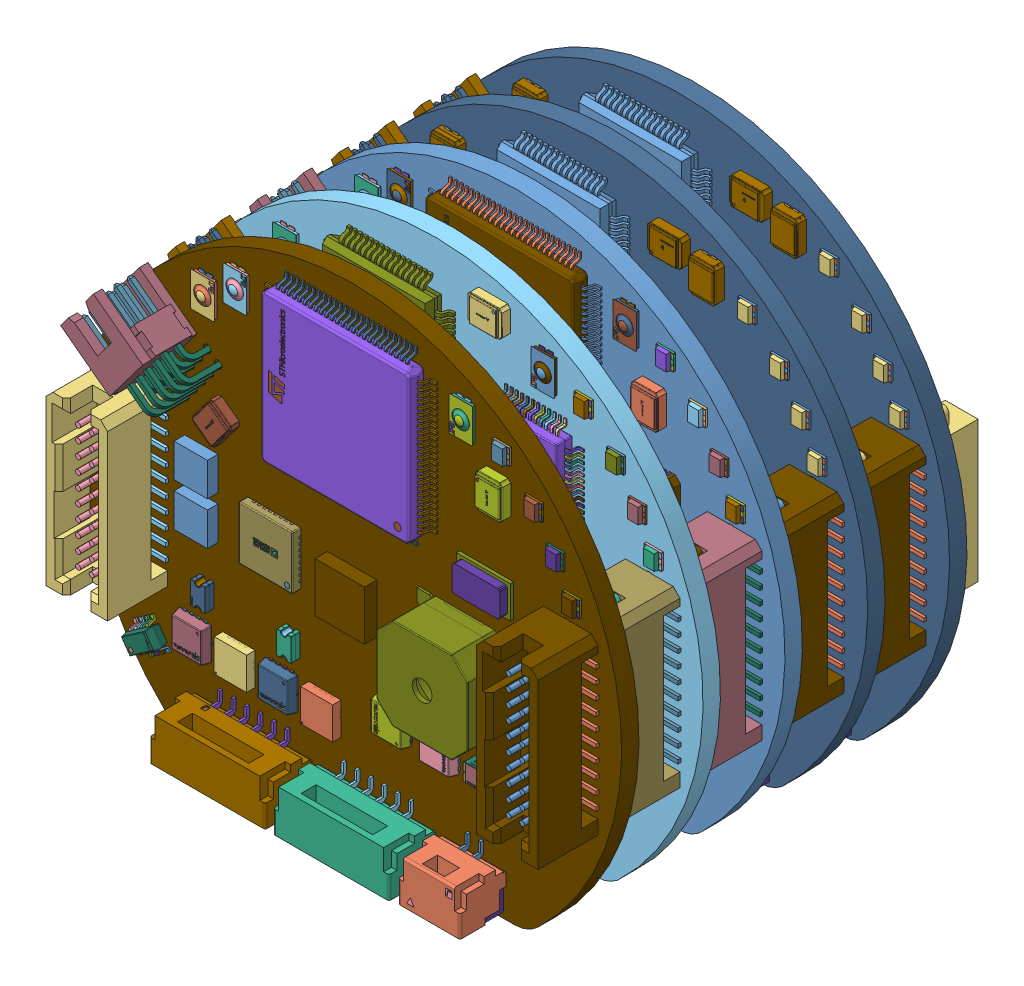
SolidWorks assembly ASSY_HYDRA_MASTER, configuration Default. Lengths in mm. (continued)
Components (placement in the parent): (continued)
- HYDRA_V4_RECOVERY-1: HYDRA_V4_RECOVERY [Default] at (-0.0049 -0.0019 15.2232) size (50.1 44.1 11.77) (continued)
  - Open CASCADE STEP translator 7.5 3383-1: Open CASCADE STEP translator 7.5 3383 [Default] at origin size (2 3 0.57)
  - Open CASCADE STEP translator 7.5 3384-1: Open CASCADE STEP translator 7.5 3384 [Default] at origin size (2.2 3.2 0.32)
  - Open CASCADE STEP translator 7.5 3385-1: Open CASCADE STEP translator 7.5 3385 [Default] at origin size (0.46 0.93 0.01)
  - Open CASCADE STEP translator 7.5 3386-1: Open CASCADE STEP translator 7.5 3386 [Default] at origin size (1.6 1.5 0.2)
  - Open CASCADE STEP translator 7.5 3387-1: Open CASCADE STEP translator 7.5 3387 [Default] at origin size (1.6 1.4 0.19)
  - Open CASCADE STEP translator 7.5 3388-1: Open CASCADE STEP translator 7.5 3388 [Default] at origin size (1.1 1.5 0.36)
  - Open CASCADE STEP translator 7.5 3389-1: Open CASCADE STEP translator 7.5 3389 [Default] at origin size (1.6 1.5 0.2)
  - Open CASCADE STEP translator 7.5 3390-1: Open CASCADE STEP translator 7.5 3390 [Default] at origin size (1.6 1.4 0.19)
  - Open CASCADE STEP translator 7.5 3391-1: Open CASCADE STEP translator 7.5 3391 [Default] at origin size (1.1 1.5 0.36)
  - Open CASCADE STEP translator 7.5 3392-1: Open CASCADE STEP translator 7.5 3392 [Default] at origin size (1.6 1.5 0.2)
  - Open CASCADE STEP translator 7.5 3393-1: Open CASCADE STEP translator 7.5 3393 [Default] at origin size (1.6 1.4 0.19)
  - Open CASCADE STEP translator 7.5 3394-1: Open CASCADE STEP translator 7.5 3394 [Default] at origin size (1.1 1.5 0.36)
  - Open CASCADE STEP translator 7.5 3395-1: Open CASCADE STEP translator 7.5 3395 [Default] at origin size (5.72 15.88 6.73)
  - Open CASCADE STEP translator 7.5 3396-1: Open CASCADE STEP translator 7.5 3396 [Default] at origin size (1.78 12.7 4.01)
  - Open CASCADE STEP translator 7.5 3397-1: Open CASCADE STEP translator 7.5 3397 [Default] at origin size (5.84 12.7 0.83)
  - Open CASCADE STEP translator 7.5 3398-1: Open CASCADE STEP translator 7.5 3398 [Default] at origin size (5.72 15.88 6.73)
  - Open CASCADE STEP translator 7.5 3399-1: Open CASCADE STEP translator 7.5 3399 [Default] at origin size (1.78 12.7 4.01)
  - Open CASCADE STEP translator 7.5 3400-1: Open CASCADE STEP translator 7.5 3400 [Default] at origin size (5.84 12.7 0.83)
  - Open CASCADE STEP translator 7.5 3401-1: Open CASCADE STEP translator 7.5 3401 [Default] at origin size (3.68 15.88 5.84)
  - Open CASCADE STEP translator 7.5 3402-1: Open CASCADE STEP translator 7.5 3402 [Default] at origin size (4.09 12.7 1.18)
  - Open CASCADE STEP translator 7.5 3403-1: Open CASCADE STEP translator 7.5 3403 [Default] at origin size (3.68 15.88 5.84)
  - Open CASCADE STEP translator 7.5 3404-1: Open CASCADE STEP translator 7.5 3404 [Default] at origin size (4.09 12.7 1.18)
- HYDRA_V4_POWER-1: HYDRA_V4_POWER [Default] at (-0.0043 -0.002 -7.6116) size (50.15 44.15 11.77)
  - Board-1: Board [Default] at origin size (50.15 44.15 1.61)
    - Open CASCADE STEP translator 7.5 2754.1.1-1: Open CASCADE STEP translator 7.5 2754.1.1 [Default] at (0 0 -1.6116) size (50.15 44.15 1.61)
  - J8-1: J8 [Default] at origin size (8.25 4.85 4.36)
    - Conn_JST_SM04B-GHS-TB_LF_SN_eec-1: Conn_JST_SM04B-GHS-TB_LF_SN_eec [Default] at (6.125 -14.4749 0.1) x (1 0 0) z (0 -1 0) size (8.25 4.36 4.85)
      - body-1: body [Default] at origin size (8.25 4.25 4.05)
      - Pins-1: Pins [Default] at origin size (7.65 2.05 4.85)
      - New Marking-1: New Marking [Default] at (-5.7821 4.251 3.7193) x (1 0 0) z (0 -1 0) size (0.46 0.67 0)
      - JST Logo-1: JST Logo [Default] at (14.4297 4.25 10.8095) x (1 0 0) z (0 1 0) size (1.76 0.68 0.01)
  - J7-1: J7 [Default] at origin size (9.7 4.86 4.36)
    - Conn_JST_SM05B-GHS-TB_LF_SN_eec-1: Conn_JST_SM05B-GHS-TB_LF_SN_eec [Default] at (11.5 -16.5 0) size (9.7 4.86 4.36)
      - 1-1: 1 [Default] at (4.75 2.025 0.1) x (1 0 0) z (0 -1 0) size (9.7 4.36 4.86)
        - 1_2-1: 1_2 [Default] at origin size (5.2 1.05 4.44)
        - SM05B-GHS-TB-1: SM05B-GHS-TB [Default] at origin size (9.7 4.26 4.06)
        - 2_2-1: 2_2 [Default] at origin size (8.9 2.05 2.2)
      - JST Logo adjustable-1: JST Logo adjustable [Default] at (-0.5885 2.016 5.7361) x (-1 0 0) z (0 1 0) size (0.68 0.81 0.01)
  - D5-1: D5 [Default] at origin size (1.6 1.5 0.55)
    - 150066xx54050-1: 150066xx54050 [Default] at (20.5 9.5 0) x (0 1 0) z (0 0 1) size (1.5 1.6 0.55)
      - body_2-1: body_2 [Default] at origin size (1.5 1.6 0.2)
      - Pads-1: Pads [Default] at origin size (1.4 1.6 0.19)
      - Dome-1: Dome [Default] x (0 -1 0) z (0 0 1) size (1.1 1.5 0.36)
  - D1-1: D1 [Default] at origin size (1.6 1.5 0.55)
    - 150066xx54050-1: 150066xx54050 [Default] at (19 12.5 0) x (0 1 0) z (0 0 1) size (1.5 1.6 0.55)
      - body_2-1: body_2 [Default] at origin size (1.5 1.6 0.2)
      - Pads-1: Pads [Default] at origin size (1.4 1.6 0.19)
      - Dome-1: Dome [Default] x (0 -1 0) z (0 0 1) size (1.1 1.5 0.36)
  - U14-1: U14 [Default] at origin size (4.5 6.6 1.15)
    - 7393011952-1: 7393011952 [Default] at (-9 -10.5 -2.8116) size (4.5 6.6 1.15)
      - Extruded_2-1: Extruded_2 [Default] at origin size (4.5 6.6 1.15)
  - D4-1: D4 [Default] at origin size (1.6 1.5 0.55)
    - 150066xx54050-1: 150066xx54050 [Default] at (14 18.5 0) x (0 1 0) z (0 0 1) size (1.5 1.6 0.55)
      - body_2-1: body_2 [Default] at origin size (1.5 1.6 0.2)
      - Pads-1: Pads [Default] at origin size (1.4 1.6 0.19)
      - Dome-1: Dome [Default] x (0 -1 0) z (0 0 1) size (1.1 1.5 0.36)
  - U13_LS_1-1: U13_LS_1 [Default] at origin size (2.02 2.02 1.01)
    - IC_Texas_Instruments_LM73100RPWR_eec-1: IC_Texas_Instruments_LM73100RPWR_eec [Default] at (-14 2.5 0) x (0 -1 0) z (0 0 1) size (2.02 2.02 1.01)
      - 1_5-1: 1_5 [Default] at origin size (2 2 0.1)
      - 2_6-1: 2_6 [Default] at origin size (2.02 2.02 0.99)
      - Texas Logo Yury-1: Texas Logo Yury [Default] at (-0.3638 0.8313 0.901) x (0 -1 0) z (0 0 1) size (0.26 0.26 0.1)
      - Texas Logo Yury - Copy-1: Texas Logo Yury - Copy [Default] at (-0.335 0.8488 0.901) x (0 -1 0) z (0 0 1) size (0.92 0.24 0.1)
  - U13_LS_0-1: U13_LS_0 [Default] at origin size (2.02 2.02 1.01)
    - IC_Texas_Instruments_LM73100RPWR_eec-1: IC_Texas_Instruments_LM73100RPWR_eec [Default] at (-14 6 0) x (0 -1 0) z (0 0 1) size (2.02 2.02 1.01)
      - 1_5-1: 1_5 [Default] at origin size (2 2 0.1)
      - 2_6-1: 2_6 [Default] at origin size (2.02 2.02 0.99)
      - Texas Logo Yury-1: Texas Logo Yury [Default] at (-0.3638 0.8313 0.901) x (0 -1 0) z (0 0 1) size (0.26 0.26 0.1)
      - Texas Logo Yury - Copy-1: Texas Logo Yury - Copy [Default] at (-0.335 0.8488 0.901) x (0 -1 0) z (0 0 1) size (0.92 0.24 0.1)
  - Y1-1: Y1 [Default] at origin size (3.23 2.53 1.01)
    - Crys_Abracon_ABM8G-12_288MHZ-18-D2Y-T3_eec-1: Crys_Abracon_ABM8G-12_288MHZ-18-D2Y-T3_eec [Default] at (7 20.5 0) x (1 0 0) z (0 0 1) size (3.23 2.53 1.01)
      - body_3-1: body_3 [Default] at origin size (3.23 2.53 1.01)
      - Termination-1: Termination [Default] at origin size (3.2 2.5 0)
      - Marking-1: Marking [Default] at (0 0 1) size (0.25 0.25 0.01)
      - Logo-1: Logo [Default] at (0 0 1) size (1.21 0.73 0.02)
  - U13_LS_2-1: U13_LS_2 [Default] at origin size (2.02 2.02 1.01)
    - IC_Texas_Instruments_LM73100RPWR_eec-1: IC_Texas_Instruments_LM73100RPWR_eec [Default] at (-14 -1 0) x (0 -1 0) z (0 0 1) size (2.02 2.02 1.01)
      - 1_5-1: 1_5 [Default] at origin size (2 2 0.1)
      - 2_6-1: 2_6 [Default] at origin size (2.02 2.02 0.99)
      - Texas Logo Yury-1: Texas Logo Yury [Default] at (-0.3638 0.8313 0.901) x (0 -1 0) z (0 0 1) size (0.26 0.26 0.1)
      - Texas Logo Yury - Copy-1: Texas Logo Yury - Copy [Default] at (-0.335 0.8488 0.901) x (0 -1 0) z (0 0 1) size (0.92 0.24 0.1)
  - U11-1: U11 [Default] at origin size (5.27 5.18 1.1)
    - 6442720976-1: 6442720976 [Default] at (-17.698 12.4027 -1.6116) x (-0.601815 -0.798635 0) z (0 0 -1) size (3.35 4.3 1.1)
  - U10-1: U10 [Default] at origin size (3.99 3.96 1.46)
    - IC_Texas_Instruments_TLV3502AIDCNT_eec-1: IC_Texas_Instruments_TLV3502AIDCNT_eec [Default] at (-18.5 -12.5 0) x (-0.573576 0.819152 0) z (0 0 1) size (2.8 2.9 1.46)
      - IC_BODY-1: IC_BODY [Default] at (0 0 0.15) size (1.6 2.9 1.31)
      - IC_LEG-1: IC_LEG [Default] at (-1.4 1.1375 0) x (1 0 0) z (0 -1 0) size (0.6 0.86 0.3)
      - IC_LEG-2: IC_LEG [Default] at (-1.4 0.4875 0) x (1 0 0) z (0 -1 0) size (0.6 0.86 0.3)
      - IC_LEG-3: IC_LEG [Default] at (-1.4 -0.1625 0) x (1 0 0) z (0 -1 0) size (0.6 0.86 0.3)
      - IC_LEG-4: IC_LEG [Default] at (-1.4 -0.8125 0) x (1 0 0) z (0 -1 0) size (0.6 0.86 0.3)
      - circle-1: circle [Default] at (-0.3239 0.9759 1.451) x (1 0 0) z (0 0 -1) size (0.4 0.4 0.01)
      - Texas Instruments-1: Texas Instruments [Default] at (0.5881 -1.1329 1.45) size (1.22 0.29 0.01)
      - IC_LEG_MIR3-1: IC_LEG_MIR3 [Default] at (1.4 1.1375 0) x (-1 0 0) z (0 1 0) size (0.6 0.86 0.3)
      - IC_LEG_MIR3-2: IC_LEG_MIR3 [Default] at (1.4 0.4875 0) x (-1 0 0) z (0 1 0) size (0.6 0.86 0.3)
      - IC_LEG_MIR3-3: IC_LEG_MIR3 [Default] at (1.4 -0.1625 0) x (-1 0 0) z (0 1 0) size (0.6 0.86 0.3)
      - IC_LEG_MIR3-4: IC_LEG_MIR3 [Default] at (1.4 -0.8125 0) x (-1 0 0) z (0 1 0) size (0.6 0.86 0.3)
  - U9-1: U9 [Default] at origin size (11.99 11.99 1.61)
    - 6684174704-1: 6684174704 [Default] at (-3 16.5 0) x (-1 0 0) z (0 0 1) size (11.99 11.99 1.61)
  - U7-1: U7 [Default] at origin size (3 3 1)
    - 7389152896-1: 7389152896 [Default] at (-0.5 1 0) size (3 3 1)
      - Extruded_4-1: Extruded_4 [Default] at origin size (3 3 1)
  - U6-1: U6 [Default] at origin size (3 3 1)
    - 7389152896-1: 7389152896 [Default] at (-0.5 5.5 0) size (3 3 1)
      - Extruded_4-1: Extruded_4 [Default] at origin size (3 3 1)
  - SW3-1: SW3 [Default] at origin size (2.53 3.5 1.01)
    - Switch_C&K_Components_KXT331LHS_eec-1: Switch_C&K_Components_KXT331LHS_eec [Default] at (-13.5 17.5 0) x (0 1 0) z (0 0 1) size (3.5 2.53 1.01)
      - terminals_3-1: terminals_3 [Default] at origin size (3.5 1.3 0.06)
      - body_3-1: body_3 [Default] at origin size (3.23 2.53 1.01)
      - button top-1: button top [Default] at (0 0 0.385) size (3.2 2.2 0.32)
      - logo_3-1: logo_3 [Default] at (0 0 0.41) size (0.93 0.46 0.01)
  - L2-1: L2 [Default] at origin size (3.65 3.01 2.02)
    - Ind_Vishay_IHLP1212BZER2R2M11_eec-1: Ind_Vishay_IHLP1212BZER2R2M11_eec [Default] at (-5.5 1 0) x (-1 0 0) z (0 0 1) size (3.65 3.01 2.02)
      - body_5-1: body_5 [Default] at origin size (3 3.01 2.01)
      - Pins_2-1: Pins_2 [Default] at origin size (3.65 0.5 1.6)
      - Logo_2-1: Logo_2 [Default] at (0 0 2) size (0.48 0.18 0.02)
  - L1-1: L1 [Default] at origin size (3.65 3.01 2.02)
    - Ind_Vishay_IHLP1212BZER2R2M11_eec-1: Ind_Vishay_IHLP1212BZER2R2M11_eec [Default] at (-5.5 5.5 0) x (-1 0 0) z (0 0 1) size (3.65 3.01 2.02)
      - body_5-1: body_5 [Default] at origin size (3 3.01 2.01)
      - Pins_2-1: Pins_2 [Default] at origin size (3.65 0.5 1.6)
      - Logo_2-1: Logo_2 [Default] at (0 0 2) size (0.48 0.18 0.02)
  - J6-1: J6 [Default] at origin size (10.53 10.1 7.35)
    - FTSH-105-01-F-D-RA-K-1: FTSH-105-01-F-D-RA-K [Default] at (-15.9584 11.7222 2.5) x (-0.601815 -0.798636 0) z (0 0 -1) size (6.27 8.46 7.35)
      - FTSH-105-01-F-D-RA-K_body-1: FTSH-105-01-F-D-RA-K_body [Default] at origin size (6.27 5.71 5.08)
      - FTSH-105-01-F-D-RA-K_pins1-1: FTSH-105-01-F-D-RA-K_pins1 [Default] at origin size (5.49 4.29 1.68)
      - FTSH-105-01-F-D-RA-K_pins2-1: FTSH-105-01-F-D-RA-K_pins2 [Default] at origin size (5.49 3.5 5.65)
  - D3-1: D3 [Default] at origin size (1.6 1.5 0.55)
    - 150066xx54050-1: 150066xx54050 [Default] at (17 15.5 0) x (0 1 0) z (0 0 1) size (1.5 1.6 0.55)
      - body_2-1: body_2 [Default] at origin size (1.5 1.6 0.2)
      - Pads-1: Pads [Default] at origin size (1.4 1.6 0.19)
      - Dome-1: Dome [Default] x (0 -1 0) z (0 0 1) size (1.1 1.5 0.36)
  - C14-1: C14 [Default] at origin size (3.01 3 2.01)
    - Cap_Taiyo_Yuden_EMK212BBJ226MG-T_eec-1: Cap_Taiyo_Yuden_EMK212BBJ226MG-T_eec [Default] at (-11 1 0) x (0 1 0) z (0 0 1) size (3 3.01 2.01)
      - terminals_5-1: terminals_5 [Default] at origin size (2.01 1.26 1.46)
      - body_5-1: body_5 [Default] at origin size (3 3.01 2.01)
      - logo_5-1: logo_5 [Default] at (0.1719 0.8617 1.45) size (0.67 0.05 0)
  - C10-1: C10 [Default] at origin size (3.01 3 2.01)
    - Cap_Taiyo_Yuden_EMK212BBJ226MG-T_eec-1: Cap_Taiyo_Yuden_EMK212BBJ226MG-T_eec [Default] at (2.5 5 -1.6116) x (0 -1 0) z (0 0 -1) size (3 3.01 2.01)
      - terminals_5-1: terminals_5 [Default] at origin size (2.01 1.26 1.46)
      - body_5-1: body_5 [Default] at origin size (3 3.01 2.01)
      - logo_5-1: logo_5 [Default] at (0.1719 0.8617 1.45) size (0.67 0.05 0)
  - C9-1: C9 [Default] at origin size (3.01 3 2.01)
    - Cap_Taiyo_Yuden_EMK212BBJ226MG-T_eec-1: Cap_Taiyo_Yuden_EMK212BBJ226MG-T_eec [Default] at (-11 5.5 0) x (0 1 0) z (0 0 1) size (3 3.01 2.01)
      - terminals_5-1: terminals_5 [Default] at origin size (2.01 1.26 1.46)
      - body_5-1: body_5 [Default] at origin size (3 3.01 2.01)
      - logo_5-1: logo_5 [Default] at (0.1719 0.8617 1.45) size (0.67 0.05 0)
  - C8-1: C8 [Default] at origin size (1.26 2.01 1.46)
    - Cap_Murata_GRM21BC71C106KE11L_eec-1: Cap_Murata_GRM21BC71C106KE11L_eec [Default] at (-9 5.5 0) x (0 1 0) z (0 0 1) size (2.01 1.26 1.46)
      - body_6-1: body_6 [Default] x (-1 0 0) z (0 0 1) size (1.1 1.25 1.45)
      - side-1: side [Default] at (-0.7 0.2667 0) x (-1 0 0) z (0 0 1) size (0.46 1.26 1.46)
      - side-2: side [Default] at (0.7 0.2667 1.45) x (1 0 0) z (0 0 -1) size (0.46 1.26 1.46)
      - Murata_2-1: Murata_2 [Default] at (-0.7353 -0.8898 1.447) size (0.62 0.15 0.01)
  - J3-1: J3 [Default] at origin size (13.3 13.95 7)
    - 6684174944-1: 6684174944 [Default] at (-9 -13 0) x (-1 0 0) z (0 1 0) size (13.3 7 13.95)
  - J5-1: J5 [Default] at origin size (5.84 15.88 6.73)
    - TFML-110-02-S-D-A-1: TFML-110-02-S-D-A [Default] at (20 0 0) x (0 1 0) z (1 0 0) size (15.88 6.73 5.84)
      - TFML-110-02-L-D-A_terminal-1: TFML-110-02-L-D-A_terminal [Default] at origin size (15.88 6.73 5.72)
      - TFML-110-02-L-D-L_pins-1: TFML-110-02-L-D-L_pins [Default] at origin size (12.7 4.01 1.78)
      - TFML-110-02-L-D-S-2_pins-1: TFML-110-02-L-D-S-2_pins [Default] at origin size (12.7 0.83 5.84)
  - J4-1: J4 [Default] at origin size (5.84 15.88 6.73)
    - TFML-110-02-S-D-A-1: TFML-110-02-S-D-A [Default] at (-20 0 0) x (0 1 0) z (1 0 0) size (15.88 6.73 5.84)
      - TFML-110-02-L-D-A_terminal-1: TFML-110-02-L-D-A_terminal [Default] at origin size (15.88 6.73 5.72)
      - TFML-110-02-L-D-L_pins-1: TFML-110-02-L-D-L_pins [Default] at origin size (12.7 4.01 1.78)
      - TFML-110-02-L-D-S-2_pins-1: TFML-110-02-L-D-S-2_pins [Default] at origin size (12.7 0.83 5.84)
  - J2-1: J2 [Default] at origin size (4.2 15.88 5.84)
    - SFML-110-02-L-D-A-1: SFML-110-02-L-D-A [Default] at (20 0 -1.6116) x (0 -1 0) z (1 0 0) size (15.88 5.84 4.2)
      - SFML-110-02-L-D-A_terminal-1: SFML-110-02-L-D-A_terminal [Default] at origin size (15.88 5.84 3.68)
      - C-10-02-D-L_pins-1: C-10-02-D-L_pins [Default] at origin size (12.7 1.18 4.09)
  - J1-1: J1 [Default] at origin size (4.2 15.88 5.84)
    - SFML-110-02-L-D-A-1: SFML-110-02-L-D-A [Default] at (-20 0 -1.6116) x (0 -1 0) z (1 0 0) size (15.88 5.84 4.2)
      - SFML-110-02-L-D-A_terminal-1: SFML-110-02-L-D-A_terminal [Default] at origin size (15.88 5.84 3.68)
      - C-10-02-D-L_pins-1: C-10-02-D-L_pins [Default] at origin size (12.7 1.18 4.09)
  - SW1-1: SW1 [Default] at origin size (2.53 3.5 1.01)
    - Switch_C&K_Components_KXT331LHS_eec-1: Switch_C&K_Components_KXT331LHS_eec [Default] at (10.5 19.5 0) x (0 -1 0) z (0 0 1) size (3.5 2.53 1.01)
      - terminals_3-1: terminals_3 [Default] at origin size (3.5 1.3 0.06)
      - body_3-1: body_3 [Default] at origin size (3.23 2.53 1.01)
      - button top-1: button top [Default] at (0 0 0.385) size (3.2 2.2 0.32)
      - logo_3-1: logo_3 [Default] at (0 0 0.41) size (0.93 0.46 0.01)
- HYDRA_V4_POWER-2: HYDRA_V4_POWER [Default] at (-0.0043 -0.002 -15.2232) size (50.15 44.15 11.77)
  - Board-1: Board [Default] at origin size (50.15 44.15 1.61)
    - Open CASCADE STEP translator 7.5 2754.1.1-1: Open CASCADE STEP translator 7.5 2754.1.1 [Default] at (0 0 -1.6116) size (50.15 44.15 1.61)
  - J8-1: J8 [Default] at origin size (8.25 4.85 4.36)
    - Conn_JST_SM04B-GHS-TB_LF_SN_eec-1: Conn_JST_SM04B-GHS-TB_LF_SN_eec [Default] at (6.125 -14.4749 0.1) x (1 0 0) z (0 -1 0) size (8.25 4.36 4.85)
      - body-1: body [Default] at origin size (8.25 4.25 4.05)
      - Pins-1: Pins [Default] at origin size (7.65 2.05 4.85)
      - New Marking-1: New Marking [Default] at (-5.7821 4.251 3.7193) x (1 0 0) z (0 -1 0) size (0.46 0.67 0)
      - JST Logo-1: JST Logo [Default] at (14.4297 4.25 10.8095) x (1 0 0) z (0 1 0) size (1.76 0.68 0.01)
  - J7-1: J7 [Default] at origin size (9.7 4.86 4.36)
    - Conn_JST_SM05B-GHS-TB_LF_SN_eec-1: Conn_JST_SM05B-GHS-TB_LF_SN_eec [Default] at (11.5 -16.5 0) size (9.7 4.86 4.36)
      - 1-1: 1 [Default] at (4.75 2.025 0.1) x (1 0 0) z (0 -1 0) size (9.7 4.36 4.86)
        - 1_2-1: 1_2 [Default] at origin size (5.2 1.05 4.44)
        - SM05B-GHS-TB-1: SM05B-GHS-TB [Default] at origin size (9.7 4.26 4.06)
        - 2_2-1: 2_2 [Default] at origin size (8.9 2.05 2.2)
      - JST Logo adjustable-1: JST Logo adjustable [Default] at (-0.5885 2.016 5.7361) x (-1 0 0) z (0 1 0) size (0.68 0.81 0.01)
  - D5-1: D5 [Default] at origin size (1.6 1.5 0.55)
    - 150066xx54050-1: 150066xx54050 [Default] at (20.5 9.5 0) x (0 1 0) z (0 0 1) size (1.5 1.6 0.55)
      - body_2-1: body_2 [Default] at origin size (1.5 1.6 0.2)
      - Pads-1: Pads [Default] at origin size (1.4 1.6 0.19)
      - Dome-1: Dome [Default] x (0 -1 0) z (0 0 1) size (1.1 1.5 0.36)
  - D1-1: D1 [Default] at origin size (1.6 1.5 0.55)
    - 150066xx54050-1: 150066xx54050 [Default] at (19 12.5 0) x (0 1 0) z (0 0 1) size (1.5 1.6 0.55)
      - body_2-1: body_2 [Default] at origin size (1.5 1.6 0.2)
      - Pads-1: Pads [Default] at origin size (1.4 1.6 0.19)
      - Dome-1: Dome [Default] x (0 -1 0) z (0 0 1) size (1.1 1.5 0.36)
  - U14-1: U14 [Default] at origin size (4.5 6.6 1.15)
    - 7393011952-1: 7393011952 [Default] at (-9 -10.5 -2.8116) size (4.5 6.6 1.15)
      - Extruded_2-1: Extruded_2 [Default] at origin size (4.5 6.6 1.15)
  - D4-1: D4 [Default] at origin size (1.6 1.5 0.55)
    - 150066xx54050-1: 150066xx54050 [Default] at (14 18.5 0) x (0 1 0) z (0 0 1) size (1.5 1.6 0.55)
      - body_2-1: body_2 [Default] at origin size (1.5 1.6 0.2)
      - Pads-1: Pads [Default] at origin size (1.4 1.6 0.19)
      - Dome-1: Dome [Default] x (0 -1 0) z (0 0 1) size (1.1 1.5 0.36)
  - U13_LS_1-1: U13_LS_1 [Default] at origin size (2.02 2.02 1.01)
    - IC_Texas_Instruments_LM73100RPWR_eec-1: IC_Texas_Instruments_LM73100RPWR_eec [Default] at (-14 2.5 0) x (0 -1 0) z (0 0 1) size (2.02 2.02 1.01)
      - 1_5-1: 1_5 [Default] at origin size (2 2 0.1)
      - 2_6-1: 2_6 [Default] at origin size (2.02 2.02 0.99)
      - Texas Logo Yury-1: Texas Logo Yury [Default] at (-0.3638 0.8313 0.901) x (0 -1 0) z (0 0 1) size (0.26 0.26 0.1)
      - Texas Logo Yury - Copy-1: Texas Logo Yury - Copy [Default] at (-0.335 0.8488 0.901) x (0 -1 0) z (0 0 1) size (0.92 0.24 0.1)
  - U13_LS_0-1: U13_LS_0 [Default] at origin size (2.02 2.02 1.01)
    - IC_Texas_Instruments_LM73100RPWR_eec-1: IC_Texas_Instruments_LM73100RPWR_eec [Default] at (-14 6 0) x (0 -1 0) z (0 0 1) size (2.02 2.02 1.01)
      - 1_5-1: 1_5 [Default] at origin size (2 2 0.1)
      - 2_6-1: 2_6 [Default] at origin size (2.02 2.02 0.99)
      - Texas Logo Yury-1: Texas Logo Yury [Default] at (-0.3638 0.8313 0.901) x (0 -1 0) z (0 0 1) size (0.26 0.26 0.1)
      - Texas Logo Yury - Copy-1: Texas Logo Yury - Copy [Default] at (-0.335 0.8488 0.901) x (0 -1 0) z (0 0 1) size (0.92 0.24 0.1)
  - Y1-1: Y1 [Default] at origin size (3.23 2.53 1.01)
    - Crys_Abracon_ABM8G-12_288MHZ-18-D2Y-T3_eec-1: Crys_Abracon_ABM8G-12_288MHZ-18-D2Y-T3_eec [Default] at (7 20.5 0) x (1 0 0) z (0 0 1) size (3.23 2.53 1.01)
      - body_3-1: body_3 [Default] at origin size (3.23 2.53 1.01)
      - Termination-1: Termination [Default] at origin size (3.2 2.5 0)
      - Marking-1: Marking [Default] at (0 0 1) size (0.25 0.25 0.01)
      - Logo-1: Logo [Default] at (0 0 1) size (1.21 0.73 0.02)
  - U13_LS_2-1: U13_LS_2 [Default] at origin size (2.02 2.02 1.01)
    - IC_Texas_Instruments_LM73100RPWR_eec-1: IC_Texas_Instruments_LM73100RPWR_eec [Default] at (-14 -1 0) x (0 -1 0) z (0 0 1) size (2.02 2.02 1.01)
      - 1_5-1: 1_5 [Default] at origin size (2 2 0.1)
      - 2_6-1: 2_6 [Default] at origin size (2.02 2.02 0.99)
      - Texas Logo Yury-1: Texas Logo Yury [Default] at (-0.3638 0.8313 0.901) x (0 -1 0) z (0 0 1) size (0.26 0.26 0.1)
      - Texas Logo Yury - Copy-1: Texas Logo Yury - Copy [Default] at (-0.335 0.8488 0.901) x (0 -1 0) z (0 0 1) size (0.92 0.24 0.1)
  - U11-1: U11 [Default] at origin size (5.27 5.18 1.1)
    - 6442720976-1: 6442720976 [Default] at (-17.698 12.4027 -1.6116) x (-0.601815 -0.798635 0) z (0 0 -1) size (3.35 4.3 1.1)
  - U10-1: U10 [Default] at origin size (3.99 3.96 1.46)
    - IC_Texas_Instruments_TLV3502AIDCNT_eec-1: IC_Texas_Instruments_TLV3502AIDCNT_eec [Default] at (-18.5 -12.5 0) x (-0.573576 0.819152 0) z (0 0 1) size (2.8 2.9 1.46)
      - IC_BODY-1: IC_BODY [Default] at (0 0 0.15) size (1.6 2.9 1.31)
      - IC_LEG-1: IC_LEG [Default] at (-1.4 1.1375 0) x (1 0 0) z (0 -1 0) size (0.6 0.86 0.3)
      - IC_LEG-2: IC_LEG [Default] at (-1.4 0.4875 0) x (1 0 0) z (0 -1 0) size (0.6 0.86 0.3)
      - IC_LEG-3: IC_LEG [Default] at (-1.4 -0.1625 0) x (1 0 0) z (0 -1 0) size (0.6 0.86 0.3)
      - IC_LEG-4: IC_LEG [Default] at (-1.4 -0.8125 0) x (1 0 0) z (0 -1 0) size (0.6 0.86 0.3)
      - circle-1: circle [Default] at (-0.3239 0.9759 1.451) x (1 0 0) z (0 0 -1) size (0.4 0.4 0.01)
      - Texas Instruments-1: Texas Instruments [Default] at (0.5881 -1.1329 1.45) size (1.22 0.29 0.01)
      - IC_LEG_MIR3-1: IC_LEG_MIR3 [Default] at (1.4 1.1375 0) x (-1 0 0) z (0 1 0) size (0.6 0.86 0.3)
      - IC_LEG_MIR3-2: IC_LEG_MIR3 [Default] at (1.4 0.4875 0) x (-1 0 0) z (0 1 0) size (0.6 0.86 0.3)
      - IC_LEG_MIR3-3: IC_LEG_MIR3 [Default] at (1.4 -0.1625 0) x (-1 0 0) z (0 1 0) size (0.6 0.86 0.3)
      - IC_LEG_MIR3-4: IC_LEG_MIR3 [Default] at (1.4 -0.8125 0) x (-1 0 0) z (0 1 0) size (0.6 0.86 0.3)
  - U9-1: U9 [Default] at origin size (11.99 11.99 1.61)
    - 6684174704-1: 6684174704 [Default] at (-3 16.5 0) x (-1 0 0) z (0 0 1) size (11.99 11.99 1.61)
  - U7-1: U7 [Default] at origin size (3 3 1)
    - 7389152896-1: 7389152896 [Default] at (-0.5 1 0) size (3 3 1)
      - Extruded_4-1: Extruded_4 [Default] at origin size (3 3 1)
  - U6-1: U6 [Default] at origin size (3 3 1)
    - 7389152896-1: 7389152896 [Default] at (-0.5 5.5 0) size (3 3 1)
      - Extruded_4-1: Extruded_4 [Default] at origin size (3 3 1)
  - SW3-1: SW3 [Default] at origin size (2.53 3.5 1.01)
    - Switch_C&K_Components_KXT331LHS_eec-1: Switch_C&K_Components_KXT331LHS_eec [Default] at (-13.5 17.5 0) x (0 1 0) z (0 0 1) size (3.5 2.53 1.01)
      - terminals_3-1: terminals_3 [Default] at origin size (3.5 1.3 0.06)
      - body_3-1: body_3 [Default] at origin size (3.23 2.53 1.01)
      - button top-1: button top [Default] at (0 0 0.385) size (3.2 2.2 0.32)
      - logo_3-1: logo_3 [Default] at (0 0 0.41) size (0.93 0.46 0.01)
  - L2-1: L2 [Default] at origin size (3.65 3.01 2.02)
    - Ind_Vishay_IHLP1212BZER2R2M11_eec-1: Ind_Vishay_IHLP1212BZER2R2M11_eec [Default] at (-5.5 1 0) x (-1 0 0) z (0 0 1) size (3.65 3.01 2.02)
      - body_5-1: body_5 [Default] at origin size (3 3.01 2.01)
      - Pins_2-1: Pins_2 [Default] at origin size (3.65 0.5 1.6)
      - Logo_2-1: Logo_2 [Default] at (0 0 2) size (0.48 0.18 0.02)
  - L1-1: L1 [Default] at origin size (3.65 3.01 2.02)
    - Ind_Vishay_IHLP1212BZER2R2M11_eec-1: Ind_Vishay_IHLP1212BZER2R2M11_eec [Default] at (-5.5 5.5 0) x (-1 0 0) z (0 0 1) size (3.65 3.01 2.02)
      - body_5-1: body_5 [Default] at origin size (3 3.01 2.01)
      - Pins_2-1: Pins_2 [Default] at origin size (3.65 0.5 1.6)
      - Logo_2-1: Logo_2 [Default] at (0 0 2) size (0.48 0.18 0.02)
  - J6-1: J6 [Default] at origin size (10.53 10.1 7.35)
    - FTSH-105-01-F-D-RA-K-1: FTSH-105-01-F-D-RA-K [Default] at (-15.9584 11.7222 2.5) x (-0.601815 -0.798636 0) z (0 0 -1) size (6.27 8.46 7.35)
      - FTSH-105-01-F-D-RA-K_body-1: FTSH-105-01-F-D-RA-K_body [Default] at origin size (6.27 5.71 5.08)
      - FTSH-105-01-F-D-RA-K_pins1-1: FTSH-105-01-F-D-RA-K_pins1 [Default] at origin size (5.49 4.29 1.68)
      - FTSH-105-01-F-D-RA-K_pins2-1: FTSH-105-01-F-D-RA-K_pins2 [Default] at origin size (5.49 3.5 5.65)
  - D3-1: D3 [Default] at origin size (1.6 1.5 0.55)
    - 150066xx54050-1: 150066xx54050 [Default] at (17 15.5 0) x (0 1 0) z (0 0 1) size (1.5 1.6 0.55)
      - body_2-1: body_2 [Default] at origin size (1.5 1.6 0.2)
      - Pads-1: Pads [Default] at origin size (1.4 1.6 0.19)
      - Dome-1: Dome [Default] x (0 -1 0) z (0 0 1) size (1.1 1.5 0.36)
  - C14-1: C14 [Default] at origin size (3.01 3 2.01)
    - Cap_Taiyo_Yuden_EMK212BBJ226MG-T_eec-1: Cap_Taiyo_Yuden_EMK212BBJ226MG-T_eec [Default] at (-11 1 0) x (0 1 0) z (0 0 1) size (3 3.01 2.01)
      - terminals_5-1: terminals_5 [Default] at origin size (2.01 1.26 1.46)
      - body_5-1: body_5 [Default] at origin size (3 3.01 2.01)
      - logo_5-1: logo_5 [Default] at (0.1719 0.8617 1.45) size (0.67 0.05 0)
  - C10-1: C10 [Default] at origin size (3.01 3 2.01)
    - Cap_Taiyo_Yuden_EMK212BBJ226MG-T_eec-1: Cap_Taiyo_Yuden_EMK212BBJ226MG-T_eec [Default] at (2.5 5 -1.6116) x (0 -1 0) z (0 0 -1) size (3 3.01 2.01)
      - terminals_5-1: terminals_5 [Default] at origin size (2.01 1.26 1.46)
      - body_5-1: body_5 [Default] at origin size (3 3.01 2.01)
      - logo_5-1: logo_5 [Default] at (0.1719 0.8617 1.45) size (0.67 0.05 0)
  - C9-1: C9 [Default] at origin size (3.01 3 2.01)
    - Cap_Taiyo_Yuden_EMK212BBJ226MG-T_eec-1: Cap_Taiyo_Yuden_EMK212BBJ226MG-T_eec [Default] at (-11 5.5 0) x (0 1 0) z (0 0 1) size (3 3.01 2.01)
      - terminals_5-1: terminals_5 [Default] at origin size (2.01 1.26 1.46)
      - body_5-1: body_5 [Default] at origin size (3 3.01 2.01)
      - logo_5-1: logo_5 [Default] at (0.1719 0.8617 1.45) size (0.67 0.05 0)
  - C8-1: C8 [Default] at origin size (1.26 2.01 1.46)
    - Cap_Murata_GRM21BC71C106KE11L_eec-1: Cap_Murata_GRM21BC71C106KE11L_eec [Default] at (-9 5.5 0) x (0 1 0) z (0 0 1) size (2.01 1.26 1.46)
      - body_6-1: body_6 [Default] x (-1 0 0) z (0 0 1) size (1.1 1.25 1.45)
      - side-1: side [Default] at (-0.7 0.2667 0) x (-1 0 0) z (0 0 1) size (0.46 1.26 1.46)
      - side-2: side [Default] at (0.7 0.2667 1.45) x (1 0 0) z (0 0 -1) size (0.46 1.26 1.46)
      - Murata_2-1: Murata_2 [Default] at (-0.7353 -0.8898 1.447) size (0.62 0.15 0.01)
  - J3-1: J3 [Default] at origin size (13.3 13.95 7)
    - 6684174944-1: 6684174944 [Default] at (-9 -13 0) x (-1 0 0) z (0 1 0) size (13.3 7 13.95)
  - J5-1: J5 [Default] at origin size (5.84 15.88 6.73)
    - TFML-110-02-S-D-A-1: TFML-110-02-S-D-A [Default] at (20 0 0) x (0 1 0) z (1 0 0) size (15.88 6.73 5.84)
      - TFML-110-02-L-D-A_terminal-1: TFML-110-02-L-D-A_terminal [Default] at origin size (15.88 6.73 5.72)
      - TFML-110-02-L-D-L_pins-1: TFML-110-02-L-D-L_pins [Default] at origin size (12.7 4.01 1.78)
      - TFML-110-02-L-D-S-2_pins-1: TFML-110-02-L-D-S-2_pins [Default] at origin size (12.7 0.83 5.84)
  - J4-1: J4 [Default] at origin size (5.84 15.88 6.73)
    - TFML-110-02-S-D-A-1: TFML-110-02-S-D-A [Default] at (-20 0 0) x (0 1 0) z (1 0 0) size (15.88 6.73 5.84)
      - TFML-110-02-L-D-A_terminal-1: TFML-110-02-L-D-A_terminal [Default] at origin size (15.88 6.73 5.72)
      - TFML-110-02-L-D-L_pins-1: TFML-110-02-L-D-L_pins [Default] at origin size (12.7 4.01 1.78)
      - TFML-110-02-L-D-S-2_pins-1: TFML-110-02-L-D-S-2_pins [Default] at origin size (12.7 0.83 5.84)
  - J2-1: J2 [Default] at origin size (4.2 15.88 5.84)
    - SFML-110-02-L-D-A-1: SFML-110-02-L-D-A [Default] at (20 0 -1.6116) x (0 -1 0) z (1 0 0) size (15.88 5.84 4.2)
      - SFML-110-02-L-D-A_terminal-1: SFML-110-02-L-D-A_terminal [Default] at origin size (15.88 5.84 3.68)
      - C-10-02-D-L_pins-1: C-10-02-D-L_pins [Default] at origin size (12.7 1.18 4.09)
  - J1-1: J1 [Default] at origin size (4.2 15.88 5.84)
    - SFML-110-02-L-D-A-1: SFML-110-02-L-D-A [Default] at (-20 0 -1.6116) x (0 -1 0) z (1 0 0) size (15.88 5.84 4.2)
      - SFML-110-02-L-D-A_terminal-1: SFML-110-02-L-D-A_terminal [Default] at origin size (15.88 5.84 3.68)
      - C-10-02-D-L_pins-1: C-10-02-D-L_pins [Default] at origin size (12.7 1.18 4.09)
  - SW1-1: SW1 [Default] at origin size (2.53 3.5 1.01)
    - Switch_C&K_Components_KXT331LHS_eec-1: Switch_C&K_Components_KXT331LHS_eec [Default] at (10.5 19.5 0) x (0 -1 0) z (0 0 1) size (3.5 2.53 1.01)
      - terminals_3-1: terminals_3 [Default] at origin size (3.5 1.3 0.06)
      - body_3-1: body_3 [Default] at origin size (3.23 2.53 1.01)
      - button top-1: button top [Default] at (0 0 0.385) size (3.2 2.2 0.32)
      - logo_3-1: logo_3 [Default] at (0 0 0.41) size (0.93 0.46 0.01)
Mates (geometry in assembly coordinates):
- Concentric1: concentric aligned: cylinder of HYDRA_V4_NAV-1/Open CASCADE STEP translator 7.5 734-1 through (-0.0048 -0.002 -1.6116) axis (0 0 -1) radius 25.0019; cylinder of HYDRA_V4_LINK_V2-1/Open CASCADE STEP translator 7.5 1-1 through (-0.0048 -0.002 6) axis (0 0 -1) radius 25.0009
- Parallel1: parallel aligned: plane of HYDRA_V4_NAV-1/Open CASCADE STEP translator 7.5 1306-1 through (-22.8575 -7.9375 5.588) normal (0 -1 0); plane of HYDRA_V4_LINK_V2-1/Open CASCADE STEP translator 7.5 731-1 through (-22.8599 -7.9391 13.1996) normal (0 -1 0)
- Distance3: distance = 6 mm anti-aligned: plane of HYDRA_V4_LINK_V2-1/Open CASCADE STEP translator 7.5 1-1 through (-0.0148 -0.2108 6) normal (0 0 -1); plane of HYDRA_V4_NAV-1/Open CASCADE STEP translator 7.5 734-1 through (0.001 -0.2558 0) normal (0 0 1)
- Concentric2: concentric aligned: cylinder of HYDRA_V4_LINK_V2-1/Open CASCADE STEP translator 7.5 1-1 through (-0.0048 -0.002 6) axis (0 0 -1) radius 25.0009; cylinder of HYDRA_V4_RECOVERY-1/Open CASCADE STEP translator 7.5 2755-1 through (-0.0048 -0.002 13.6116) axis (0 0 -1) radius 25.0501
- Parallel2: parallel aligned: plane of HYDRA_V4_LINK_V2-1/Open CASCADE STEP translator 7.5 731-1 through (-22.8599 -7.9391 13.1996) normal (0 -1 0); plane of HYDRA_V4_RECOVERY-1/Open CASCADE STEP translator 7.5 3398-1 through (-22.8624 -7.9394 20.8112) normal (0 -1 0)
- Distance4: distance = 6 mm anti-aligned: plane of HYDRA_V4_RECOVERY-1/Open CASCADE STEP translator 7.5 2755-1 through (-0.0031 -0.4141 13.6116) normal (0 0 -1); plane of HYDRA_V4_LINK_V2-1/Open CASCADE STEP translator 7.5 1-1 through (-0.0148 -0.2108 7.6116) normal (0 0 1)
- Concentric3: concentric aligned: cylinder of HYDRA_V4_NAV-1/Open CASCADE STEP translator 7.5 734-1 through (-0.0048 -0.002 -1.6116) axis (0 0 -1) radius 25.0019; cylinder of HYDRA_V4_POWER-1/Board-1/Open CASCADE STEP translator 7.5 2754.1.1-1 through (-0.0048 -0.002 -9.2232) axis (0 0 -1) radius 25.0756
- Parallel3: parallel aligned: plane of HYDRA_V4_NAV-1/Open CASCADE STEP translator 7.5 1306-1 through (-22.8575 -7.9375 5.588) normal (0 -1 0); plane of HYDRA_V4_POWER-1/J4-1/TFML-110-02-S-D-A-1/TFML-110-02-L-D-A_terminal-1 through (-22.8618 -7.9395 -2.0236) normal (0 -1 0)
- Distance5: distance = 6 mm anti-aligned: plane of HYDRA_V4_NAV-1/Open CASCADE STEP translator 7.5 734-1 through (0.001 -0.2558 -1.6116) normal (0 0 -1); plane of HYDRA_V4_POWER-1/Board-1/Open CASCADE STEP translator 7.5 2754.1.1-1 through (-0.0414 -0.2017 -7.6116) normal (0 0 1)
- Concentric4: concentric aligned: cylinder of HYDRA_V4_POWER-1/Board-1/Open CASCADE STEP translator 7.5 2754.1.1-1 through (-0.0048 -0.002 -9.2232) axis (0 0 -1) radius 25.0756; cylinder of HYDRA_V4_POWER-2/Board-1/Open CASCADE STEP translator 7.5 2754.1.1-1 through (-0.0048 -0.002 -16.8348) axis (0 0 -1) radius 25.0756
- Parallel4: parallel aligned: plane of HYDRA_V4_POWER-1/J4-1/TFML-110-02-S-D-A-1/TFML-110-02-L-D-A_terminal-1 through (-22.8618 -7.9395 -2.0236) normal (0 -1 0); plane of HYDRA_V4_POWER-2/J4-1/TFML-110-02-S-D-A-1/TFML-110-02-L-D-A_terminal-1 through (-22.8618 -7.9395 -9.6352) normal (0 -1 0)
- Distance6: distance = 6 mm anti-aligned: plane of HYDRA_V4_POWER-1/Board-1/Open CASCADE STEP translator 7.5 2754.1.1-1 through (-0.0414 -0.2017 -9.2232) normal (0 0 -1); plane of HYDRA_V4_POWER-2/Board-1/Open CASCADE STEP translator 7.5 2754.1.1-1 through (-0.0414 -0.2017 -15.2232) normal (0 0 1)
